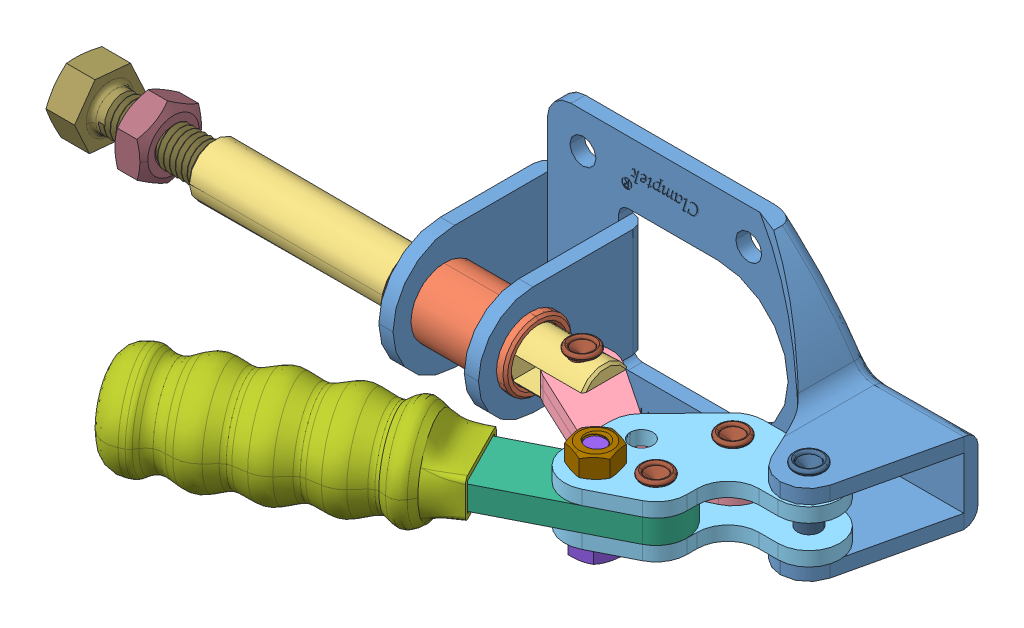
SolidWorks assembly Clamp GH-302-FM (Clamptek CH-302-FM), configuration Default. Lengths in mm.
Overall size (165.14 56.02 86.64).
17 component instances, 13 part files, 33 mates.
Components (placement in the parent):
- Основа^Clamp GH-302-FM (Clamptek CH-302-FM)-1: Основа^Clamp GH-302-FM (Clamptek CH-302-FM) [Default] at origin size (90.9 56.02 35.6) (virtual)
- Кольцо^Clamp GH-302-FM (Clamptek CH-302-FM)-1: Кольцо^Clamp GH-302-FM (Clamptek CH-302-FM) [Default] at (-54.2789 -11.6012 17.5543) size (25.5 17 17) (virtual)
- Поршинь^Clamp GH-302-FM (Clamptek CH-302-FM)-1: Поршинь^Clamp GH-302-FM (Clamptek CH-302-FM) [Default] at (-54.2917 -11.6012 17.5543) size (83 10.87 10.86) (virtual)
- Колено^Clamp GH-302-FM (Clamptek CH-302-FM)-1: Колено^Clamp GH-302-FM (Clamptek CH-302-FM) [Default] at (-54.1752 -11.6012 17.4501) x (0.999865 0 0.016412) z (-0.016412 0 0.999865) size (44.3 2.5 20.11) (virtual)
- Колено^Clamp GH-302-FM (Clamptek CH-302-FM)-2: Колено^Clamp GH-302-FM (Clamptek CH-302-FM) [Default] at (-54.1752 -9.1012 17.4501) x (0.999865 0 0.016412) z (-0.016412 0 0.999865) size (44.3 2.5 20.11) (virtual)
- Колено2^Clamp GH-302-FM (Clamptek CH-302-FM)-1: Колено2^Clamp GH-302-FM (Clamptek CH-302-FM) [Default] at (-54.4794 -11.6012 19.3226) x (0.99947 0 -0.032538) z (0.032538 0 0.99947) size (39.16 3 32.18) (virtual)
- Колено2^Clamp GH-302-FM (Clamptek CH-302-FM)-2: Колено2^Clamp GH-302-FM (Clamptek CH-302-FM) [Default] at (-54.4794 -3.6012 19.3226) x (0.99947 0 -0.032538) z (0.032538 0 0.99947) size (39.16 3 32.18) (virtual)
- Рычаг^Clamp GH-302-FM (Clamptek CH-302-FM)-1: Рычаг^Clamp GH-302-FM (Clamptek CH-302-FM) [Default] at (-54.4794 -11.6012 19.3226) x (0.99947 0 -0.032538) z (0.032538 0 0.99947) size (81.85 5 45.18) (virtual)
- Рукаять^Clamp GH-302-FM (Clamptek CH-302-FM)-1: Рукаять^Clamp GH-302-FM (Clamptek CH-302-FM) [Default] at (-54.4794 -11.1014 19.3226) x (0.99947 0 -0.032538) z (0.032538 0 0.99947) size (59.04 21.79 39.34) (virtual)
- Винт М5х15^Clamp GH-302-FM (Clamptek CH-302-FM)-2: Винт М5х15^Clamp GH-302-FM (Clamptek CH-302-FM) [Default] at (-50.7069 -11.6012 15.5048) x (0.99411 0 0.108374) z (-0.108374 0 0.99411) size (8.82 19.5 9.05) (virtual)
- Гайка М5^Clamp GH-302-FM (Clamptek CH-302-FM)-1: Гайка М5^Clamp GH-302-FM (Clamptek CH-302-FM) [Default] at (-63.6387 -11.6012 43.2355) x (0.752669 0 -0.658399) z (0.658399 0 0.752669) size (9.25 4.51 8.16) (virtual)
- Заклёпка 17мм^Clamp GH-302-FM (Clamptek CH-302-FM)-2: Заклёпка 17мм^Clamp GH-302-FM (Clamptek CH-302-FM) [Default] at (-54.2789 -11.6012 17.5543) size (9.29 19.7 8.86) (virtual)
- Заклёпка 11мм^Clamp GH-302-FM (Clamptek CH-302-FM)-3: Заклёпка 11мм^Clamp GH-302-FM (Clamptek CH-302-FM) [Default] at (-54.2917 -11.5491 17.5543) size (9.59 13.7 9.1) (virtual)
- Заклёпка 11мм^Clamp GH-302-FM (Clamptek CH-302-FM)-4: Заклёпка 11мм^Clamp GH-302-FM (Clamptek CH-302-FM) [Default] at (-22.6054 -11.6191 32.02) x (0.992409 0 0.12298) z (-0.12298 0 0.992409) size (9.59 13.7 9.1) (virtual)
- Заклёпка 11мм^Clamp GH-302-FM (Clamptek CH-302-FM)-5: Заклёпка 11мм^Clamp GH-302-FM (Clamptek CH-302-FM) [Default] at (-21.5766 -11.6191 16.82) x (0.992409 0 0.12298) z (-0.12298 0 0.992409) size (9.59 13.7 9.1) (virtual)
- Винт фиксирующий М8х50^Clamp GH-302-FM (Clamptek CH-302-FM)-1: Винт фиксирующий М8х50^Clamp GH-302-FM (Clamptek CH-302-FM) [Default] at (-60.9918 -12.1166 18.483) x (1 0 0) z (0 0.078196 0.996938) size (56.51 13.09 15.02) (virtual)
- Гайка фиксирующая М8^Clamp GH-302-FM (Clamptek CH-302-FM)-1: Гайка фиксирующая М8^Clamp GH-302-FM (Clamptek CH-302-FM) [Default] at (-62.5752 11.856 31.2079) x (1 0 0) z (0 -0.037313 -0.999304) size (6.51 15 13.33) (virtual)
Mates (geometry in assembly coordinates):
- Концентричный1: concentric: cylinder of Основа^Clamp GH-302-FM (Clamptek CH-302-FM)-1 through (-39.8419 0 24.6) axis (-1 0 0) radius 7.25; cylinder of Кольцо^Clamp GH-302-FM (Clamptek CH-302-FM)-1 through (-82.4419 0 24.6) axis (1 0 0) radius 7.2
- Совпадение1: coincident: plane of Основа^Clamp GH-302-FM (Clamptek CH-302-FM)-1 through (-79.8419 0 0) normal (-1 0 0); plane of Кольцо^Clamp GH-302-FM (Clamptek CH-302-FM)-1 through (-79.8419 0 24.6) normal (1 0 0)
- Параллельность1: parallel: plane of Основа^Clamp GH-302-FM (Clamptek CH-302-FM)-1 through (-78.7076 32.6238 0) normal (0 0 -1); plane of Кольцо^Clamp GH-302-FM (Clamptek CH-302-FM)-1 through (-54.2789 -11.6012 17.5543) normal (0 0 1)
- Концентричный2: concentric: cylinder of Кольцо^Clamp GH-302-FM (Clamptek CH-302-FM)-1 through (-56.9419 0 24.6) axis (-1 0 0) radius 5.43; cylinder of Поршинь^Clamp GH-302-FM (Clamptek CH-302-FM)-1 through (-42.8862 0 24.6) axis (-1 0 0) radius 5.43
- Концентричный3: concentric: cylinder of Поршинь^Clamp GH-302-FM (Clamptek CH-302-FM)-1 through (-47.8862 -83 24.6) axis (0 1 0) radius 2.4; cylinder of Колено^Clamp GH-302-FM (Clamptek CH-302-FM)-1 through (-47.8862 -2.5 24.6) axis (0 1 0) radius 2.4
- Совпадение3: coincident: plane of Основа^Clamp GH-302-FM (Clamptek CH-302-FM)-1 through (0 0 0) normal (0 1 0); plane of Колено^Clamp GH-302-FM (Clamptek CH-302-FM)-1 through (-16.0862 0 24.6) normal (0 1 0)
- Концентричный4: concentric: cylinder of Колено^Clamp GH-302-FM (Clamptek CH-302-FM)-1 through (-16.0862 -2.5 24.6) axis (0 1 0) radius 2.4; cylinder of Колено2^Clamp GH-302-FM (Clamptek CH-302-FM)-1 through (-16.0862 -5.5 24.6) axis (0 1 0) radius 2.4
- Концентричный5: concentric: cylinder of Основа^Clamp GH-302-FM (Clamptek CH-302-FM)-1 through (-0.0462 72 24.6) axis (0 -1 0) radius 2.4; cylinder of Колено2^Clamp GH-302-FM (Clamptek CH-302-FM)-1 through (-0.0462 -5.5 24.6) axis (0 1 0) radius 2.4
- Совпадение4: coincident: plane of Колено^Clamp GH-302-FM (Clamptek CH-302-FM)-1 through (-16.0862 -2.5 24.6) normal (0 -1 0); plane of Колено2^Clamp GH-302-FM (Clamptek CH-302-FM)-1 through (-16.0862 -2.5 24.6) normal (0 1 0)
- Концентричный6: concentric: cylinder of Колено2^Clamp GH-302-FM (Clamptek CH-302-FM)-1 through (-17.1151 -5.5 39.8) axis (0 1 0) radius 2.4; cylinder of Рычаг^Clamp GH-302-FM (Clamptek CH-302-FM)-1 through (-17.1151 -2.5 39.8) axis (0 1 0) radius 2.4
- Концентричный7: concentric: cylinder of Колено2^Clamp GH-302-FM (Clamptek CH-302-FM)-1 through (-25.5862 -5.5 44.1) axis (0 1 0) radius 2.5; cylinder of Рычаг^Clamp GH-302-FM (Clamptek CH-302-FM)-1 through (-25.5862 -2.5 44.1) axis (0 1 0) radius 2.4
- Совпадение5: coincident: plane of Колено2^Clamp GH-302-FM (Clamptek CH-302-FM)-1 through (-16.0862 -2.5 24.6) normal (0 1 0); plane of Рычаг^Clamp GH-302-FM (Clamptek CH-302-FM)-1 through (-17.1151 -2.5 39.8) normal (0 -1 0)
- Граничный угол1: limit planar angle = 2.671878 rad: plane of Основа^Clamp GH-302-FM (Clamptek CH-302-FM)-1 through (-78.7076 32.6238 0) normal (0 0 -1); plane of Рычаг^Clamp GH-302-FM (Clamptek CH-302-FM)-1 through (-14.173 -2.5 45.596) normal (0.452632 0 0.891698)
- Концентричный8: concentric: cylinder of Рычаг^Clamp GH-302-FM (Clamptek CH-302-FM)-1 through (-84.8841 -2.5 74.2) axis (0 1 0) radius 6.5; cylinder of Рукаять^Clamp GH-302-FM (Clamptek CH-302-FM)-1 through (-84.8841 2.9998 74.2) axis (0 -1 0) radius 6.5
- Совпадение8: coincident: plane of Рычаг^Clamp GH-302-FM (Clamptek CH-302-FM)-1 through (-14.173 -2.5 45.596) normal (0.452632 0 0.891698); plane of Рукаять^Clamp GH-302-FM (Clamptek CH-302-FM)-1 through (-87.738 -3.0002 82.9381) normal (-0.452632 0 -0.891698)
- Совпадение10: coincident: plane of Рычаг^Clamp GH-302-FM (Clamptek CH-302-FM)-1 through (-54.4794 0 19.3226) normal (0 -1 0); line of Рукаять^Clamp GH-302-FM (Clamptek CH-302-FM)-1 through (-95.1941 0 79.4332) axis (0.654328 0 0.756211)
- Концентричный9: concentric: cylinder of Колено2^Clamp GH-302-FM (Clamptek CH-302-FM)-1 through (-25.5862 -5.5 44.1) axis (0 1 0) radius 2.5; cylinder of Винт М5х15^Clamp GH-302-FM (Clamptek CH-302-FM)-2 through (-25.5862 9.5 44.1) axis (0 -1 0) radius 2.5
- Совпадение11: coincident: plane of Колено2^Clamp GH-302-FM (Clamptek CH-302-FM)-1 through (-16.0862 -5.5 24.6) normal (0 -1 0); plane of Винт М5х15^Clamp GH-302-FM (Clamptek CH-302-FM)-2 through (-24.1217 -5.5 39.7195) normal (0 1 0)
- Совпадение12: coincident: plane of Колено2^Clamp GH-302-FM (Clamptek CH-302-FM)-2 through (-16.0862 5.5 24.6) normal (0 1 0); plane of Гайка М5^Clamp GH-302-FM (Clamptek CH-302-FM)-1 through (-31.0441 5.5 38.2509) normal (0 -1 0)
- Концентричный10: concentric: cylinder of Колено2^Clamp GH-302-FM (Clamptek CH-302-FM)-1 through (-25.5862 -5.5 44.1) axis (0 1 0) radius 2.5; circle of Гайка М5^Clamp GH-302-FM (Clamptek CH-302-FM)-1
- Концентричный11: concentric: cylinder of Основа^Clamp GH-302-FM (Clamptek CH-302-FM)-1 through (-0.0462 72 24.6) axis (0 -1 0) radius 2.4; cylinder of Заклёпка 17мм^Clamp GH-302-FM (Clamptek CH-302-FM)-2 through (-0.0462 8.5 24.6) axis (0 -1 0) radius 2.4
- Совпадение13: coincident: plane of Основа^Clamp GH-302-FM (Clamptek CH-302-FM)-1 through (11.0538 -8.5 3) normal (0 -1 0); plane of Заклёпка 17мм^Clamp GH-302-FM (Clamptek CH-302-FM)-2 through (-0.0462 -8.5 24.6) normal (0 1 0)
- Совпадение14: coincident: point of Поршинь^Clamp GH-302-FM (Clamptek CH-302-FM)-1; plane of Заклёпка 11мм^Clamp GH-302-FM (Clamptek CH-302-FM)-3 through (-47.8862 -5.43 24.6) normal (0 1 0)
- Концентричный12: concentric: cylinder of Поршинь^Clamp GH-302-FM (Clamptek CH-302-FM)-1 through (-47.8862 -83 24.6) axis (0 1 0) radius 2.4; cylinder of Заклёпка 11мм^Clamp GH-302-FM (Clamptek CH-302-FM)-3 through (-47.8862 5.57 24.6) axis (0 -1 0) radius 2.4
- Совпадение15: coincident: plane of Колено2^Clamp GH-302-FM (Clamptek CH-302-FM)-1 through (-16.0862 -5.5 24.6) normal (0 -1 0); plane of Заклёпка 11мм^Clamp GH-302-FM (Clamptek CH-302-FM)-5 through (-16.0862 -5.5 24.6) normal (0 1 0)
- Совпадение16: coincident: plane of Колено2^Clamp GH-302-FM (Clamptek CH-302-FM)-1 through (-16.0862 -5.5 24.6) normal (0 -1 0); plane of Заклёпка 11мм^Clamp GH-302-FM (Clamptek CH-302-FM)-4 through (-17.1151 -5.5 39.8) normal (0 1 0)
- Концентричный13: concentric: cylinder of Колено2^Clamp GH-302-FM (Clamptek CH-302-FM)-1 through (-16.0862 -5.5 24.6) axis (0 1 0) radius 2.4; cylinder of Заклёпка 11мм^Clamp GH-302-FM (Clamptek CH-302-FM)-5 through (-16.0862 5.5 24.6) axis (0 -1 0) radius 2.4
- Концентричный14: concentric: cylinder of Колено2^Clamp GH-302-FM (Clamptek CH-302-FM)-1 through (-17.1151 -5.5 39.8) axis (0 1 0) radius 2.4; cylinder of Заклёпка 11мм^Clamp GH-302-FM (Clamptek CH-302-FM)-4 through (-17.1151 5.5 39.8) axis (0 -1 0) radius 2.4
- Концентричный15: concentric: cylinder of Поршинь^Clamp GH-302-FM (Clamptek CH-302-FM)-1 through (-90.8862 0 24.6) axis (-1 0 0) radius 3.4; cylinder of Винт фиксирующий М8х50^Clamp GH-302-FM (Clamptek CH-302-FM)-1 through (-97.5864 0 24.6) axis (-1 0 0) radius 4
- Концентричный16: concentric: cylinder of Винт фиксирующий М8х50^Clamp GH-302-FM (Clamptek CH-302-FM)-1 through (-97.5864 0 24.6) axis (-1 0 0) radius 4; circle of Гайка фиксирующая М8^Clamp GH-302-FM (Clamptek CH-302-FM)-1
- Граничное расстояние1: limit distance = 6.7002 mm: plane of Винт фиксирующий М8х50^Clamp GH-302-FM (Clamptek CH-302-FM)-1 through (-97.5864 0 24.6) normal (1 0 0); plane of Поршинь^Clamp GH-302-FM (Clamptek CH-302-FM)-1 through (-90.8862 0 24.6) normal (-1 0 0)
- Граничное расстояние2: limit distance = 8.2835 mm: plane of Поршинь^Clamp GH-302-FM (Clamptek CH-302-FM)-1 through (-125.8862 0 24.6) normal (-1 0 0); plane of Гайка фиксирующая М8^Clamp GH-302-FM (Clamptek CH-302-FM)-1 through (-134.1697 -11.2123 18.0209) normal (1 0 0)
- Граничное расстояние3: limit distance = 6.9167 mm: plane of Гайка фиксирующая М8^Clamp GH-302-FM (Clamptek CH-302-FM)-1 through (-140.6697 -11.2123 18.0209) normal (-1 0 0); plane of Винт фиксирующий М8х50^Clamp GH-302-FM (Clamptek CH-302-FM)-1 through (-147.5864 -12.9476 25.7661) normal (1 0 0)
